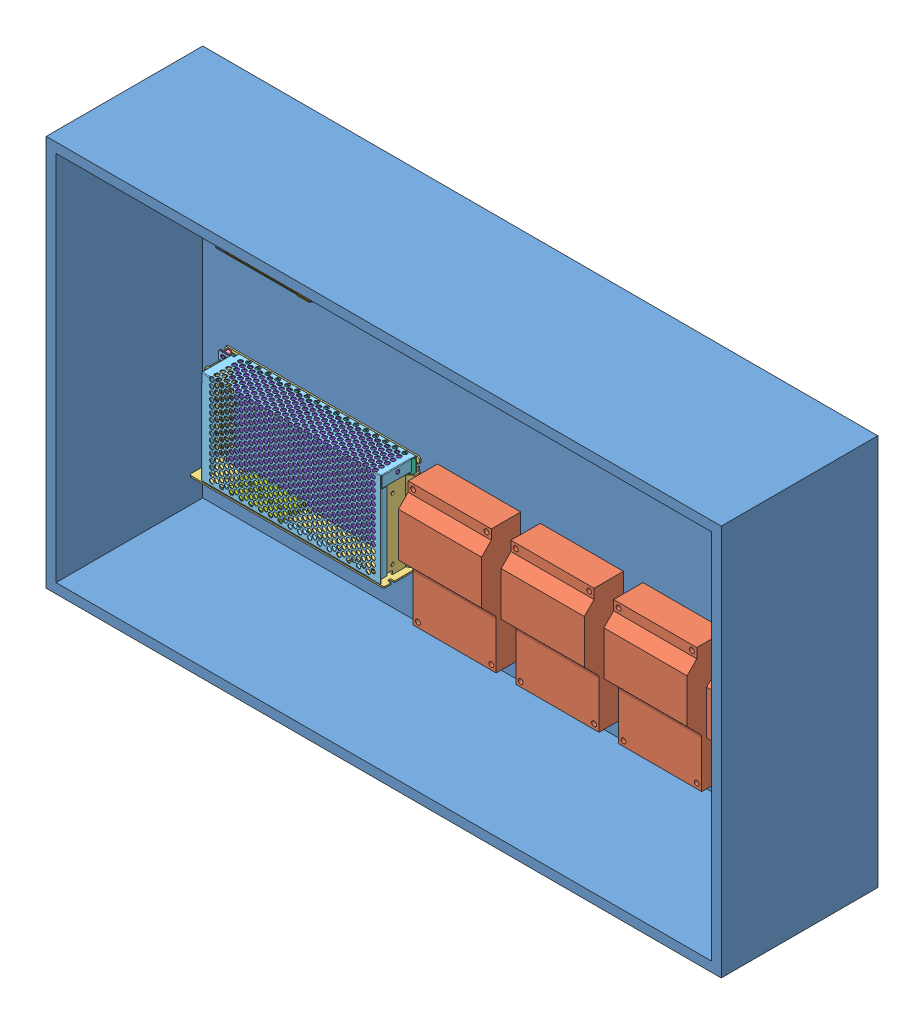
SolidWorks assembly quadro_elettrico_full, configuration Default. Lengths in mm.
Overall size (690 400 160).
33 component instances, 20 part files, 17 mates.
Components (placement in the parent):
- quadro_elettrico-1: quadro_elettrico [Default] at origin size (690 400 160)
- minitraction_power_mockup-1: minitraction_power_mockup [Default] at (-52.5 -105 10) size (85 130 40)
- SD-100C-12-1: SD-100C-12 [Default] at (-211.5 -91.125 11.5) x (1 0 0) z (0 -1 0) size (199.09 37.75 98.27)
  - SD-100C-12.stp-1: SD-100C-12.stp [Default] at origin size (199.09 37.75 98.27)
    - SD-100-20201028.stp.stp-1: SD-100-20201028.stp.stp [Default] at origin size (199.09 37.75 98.27)
      - SD-100_STP.ASM.stp-1: SD-100_STP.ASM.stp [Default] at origin size (199.09 37.75 98.27)
        - SD-100_1_ASM.ASM.stp-1: SD-100_1_ASM.ASM.stp [Default] at origin size (199 37.75 98.27)
          - 902-D-80_ASM.ASM.stp-1: 902-D-80_ASM.ASM.stp [Default] at origin size (199 37.75 97.75)
            - 902-D-119_PRT.PRT.stp-1: 902-D-119_PRT.PRT.stp [Default] at origin size (199 37.75 97.75)
            - NUT_PRT.PRT.stp-1: NUT_PRT.PRT.stp [Default] at (-111.528 -1.5 -40.7894) x (-1 0 0) z (0 1 0) size (8 6.93 6)
          - 902-T_PRT.PRT.stp-1: 902-T_PRT.PRT.stp [Default] at (96.5 36.1 -49.375) x (-1 0 0) z (0 0 -1) size (195.5 36.02 96.52)
          - MYLAR_PRT.PRT.stp-1: MYLAR_PRT.PRT.stp [Default] at (79.2081 1.5 46.5396) x (-1 0 0) z (0 -1 0) size (197 95 0.5)
          - HS2_PRT.PRT.stp-1: HS2_PRT.PRT.stp [Default] at (-64.5 -80.2586 -88.3567) x (0 0 1) z (-1 0 0) size (6.4 28 55)
          - PCB_PRT.PRT.stp-1: PCB_PRT.PRT.stp [Default] at (-189.5595 4.5 45.0362) x (1 0 0) z (0 1 0) size (194 95 1.6)
        - T44-BS1R05370120201023_STP.ASM.stp-1: T44-BS1R05370120201023_STP.ASM.stp [Default] at (-82.3888 6.1 -32.875) x (0 0 1) z (0 1 0) size (69.8 18 18.8)
          - 6_PRT.PRT.stp-1: 6_PRT.PRT.stp [Default] at origin size (7.51 7.5 3.96)
          - 2_PRT.PRT.stp-1: 2_PRT.PRT.stp [Default] at origin size (7.5 7.5 3.96)
          - 3_PRT.PRT.stp-1: 3_PRT.PRT.stp [Default] at origin size (7.51 7.5 3.96)
          - 4_PRT.PRT.stp-1: 4_PRT.PRT.stp [Default] at (0 0.8 0) size (69.8 18 18.8)
          - 5_PRT.PRT.stp-1: 5_PRT.PRT.stp [Default] at origin size (7.51 7.5 3.96)
          - 6_PRT_1.PRT.stp-1: 6_PRT_1.PRT.stp [Default] at (9.5 0 0) size (7.51 7.5 3.96)
          - 6_PRT_1_1.PRT.stp-1: 6_PRT_1_1.PRT.stp [Default] at (19 0 0) size (7.51 7.5 3.96)
          - 6_PRT_1_1_1.PRT.stp-1: 6_PRT_1_1_1.PRT.stp [Default] at (28.5 0 0) size (7.51 7.5 3.96)
- SD-25C-12-1: SD-25C-12 [Default] at (28.1917 -114.0246 17.8) size (99.05 97.03 36.06)
  - SD-25C-12.stp-1: SD-25C-12.stp [Default] at origin size (99.05 97.03 36.06)
    - RS-50_ASM_15.ASM.stp-1: RS-50_ASM_15.ASM.stp [Default] at origin size (99.05 97.03 36.06)
      - TN1_2.PRT.stp-1: TN1_2.PRT.stp [Default] at (-301.0065 335.8998 37.1723) x (0 0 -1) z (-1 0 0) size (15.25 49.25 14.66)
      - RS-50-CASE-T_21.PRT.stp-1: RS-50-CASE-T_21.PRT.stp [Default] at (0 1.5 1) size (97.05 96.6 36.06)
      - RS-50-CASE-D_28.PRT.stp-1: RS-50-CASE-D_28.PRT.stp [Default] at (-0.5 0.5 0) size (98.5 97 35)
      - RS-50-PCB_2.PRT.stp-1: RS-50-PCB_2.PRT.stp [Default] at (0 -0.6 -0.2033) size (98 95 1.6)
- minitraction_power_mockup-2: minitraction_power_mockup [Default] at (52.5 -105 10) size (85 130 40)
- minitraction_power_mockup-3: minitraction_power_mockup [Default] at (157.5 -105 10) size (85 130 40)
- minitraction_power_mockup-4: minitraction_power_mockup [Default] at (262.5 -105 10) size (85 130 40)
Mates (geometry in assembly coordinates):
- Coincidente1: coincident anti-aligned: plane of quadro_elettrico-1 through (0 0 10) normal (0 0 1); plane of minitraction_power_mockup-4 through (262.5 -105 10) normal (0 0 -1)
- Coincidente2: coincident anti-aligned: plane of quadro_elettrico-1 through (0 0 10) normal (0 0 1); plane of minitraction_power_mockup-3 through (157.5 -105 10) normal (0 0 -1)
- Coincidente3: coincident anti-aligned: plane of quadro_elettrico-1 through (0 0 10) normal (0 0 1); plane of minitraction_power_mockup-2 through (52.5 -105 10) normal (0 0 -1)
- Coincidente4: coincident anti-aligned: plane of quadro_elettrico-1 through (0 0 10) normal (0 0 1); plane of minitraction_power_mockup-1 through (-52.5 -105 10) normal (0 0 -1)
- Distanza1: distance = 20 mm anti-aligned: plane of minitraction_power_mockup-2 through (10 -40 50) normal (-1 0 0); plane of minitraction_power_mockup-1 through (-10 -40 50) normal (1 0 0)
- Coincidente6: coincident aligned: plane of minitraction_power_mockup-1 through (-95 -40 50) normal (0 1 0); plane of minitraction_power_mockup-2 through (10 -40 50) normal (0 1 0)
- Distanza2: distance = 20 mm anti-aligned: plane of minitraction_power_mockup-3 through (115 -40 50) normal (-1 0 0); plane of minitraction_power_mockup-2 through (95 -40 50) normal (1 0 0)
- Distanza3: distance = 20 mm anti-aligned: plane of minitraction_power_mockup-3 through (200 -40 50) normal (1 0 0); plane of minitraction_power_mockup-4 through (220 -40 50) normal (-1 0 0)
- Coincidente9: coincident aligned: plane of minitraction_power_mockup-3 through (115 -40 50) normal (0 1 0); plane of minitraction_power_mockup-4 through (220 -40 50) normal (0 1 0)
- Coincidente10: coincident aligned: plane of minitraction_power_mockup-2 through (10 -40 50) normal (0 1 0); plane of minitraction_power_mockup-3 through (115 -40 50) normal (0 1 0)
- Distanza4: distance = 30 mm anti-aligned: plane of minitraction_power_mockup-4 through (305 -40 50) normal (1 0 0); plane of quadro_elettrico-1 through (335 -190 160) normal (-1 0 0)
- Distanza5: distance = 20 mm anti-aligned: plane of minitraction_power_mockup-4 through (220 -170 50) normal (0 -1 0); plane of quadro_elettrico-1 through (-335 -190 160) normal (0 1 0)
- Coincidente11: coincident anti-aligned: plane of quadro_elettrico-1 through (0 0 10) normal (0 0 1); plane of SD-100C-12-1/SD-100C-12.stp-1/SD-100-20201028.stp.stp-1/SD-100_STP.ASM.stp-1/SD-100_1_ASM.ASM.stp-1/902-D-80_ASM.ASM.stp-1/902-D-119_PRT.PRT.stp-1 through (-211.5 -91.125 10) normal (0 0 -1)
- Distanza7: distance = 50 mm anti-aligned: plane of SD-100C-12-1/SD-100C-12.stp-1/SD-100-20201028.stp.stp-1/SD-100_STP.ASM.stp-1/SD-100_1_ASM.ASM.stp-1/902-D-80_ASM.ASM.stp-1/902-D-119_PRT.PRT.stp-1 through (-112 -140 10) normal (0 -1 0); plane of quadro_elettrico-1 through (-335 -190 160) normal (0 1 0)
- Distanza8: distance = 20 mm anti-aligned: plane of minitraction_power_mockup-1 through (-95 -40 50) normal (-1 0 0); plane of SD-100C-12-1/SD-100C-12.stp-1/SD-100-20201028.stp.stp-1/SD-100_STP.ASM.stp-1/SD-100_1_ASM.ASM.stp-1/902-T_PRT.PRT.stp-1 through (-115 -41.75 38.4938) normal (1 0 0)
- Distanza9: distance = 20 mm: plane of SD-25C-12-1/SD-25C-12.stp-1/RS-50_ASM_15.ASM.stp-1/RS-50-CASE-T_21.PRT.stp-1 through (-275.9748 170 12.5) normal (0 1 0); plane of quadro_elettrico-1 through (335 190 160) normal (0 -1 0)
- Coincidente12: coincident anti-aligned: plane of quadro_elettrico-1 through (0 0 10) normal (0 0 1); plane of SD-25C-12-1/SD-25C-12.stp-1/RS-50_ASM_15.ASM.stp-1/RS-50-CASE-D_28.PRT.stp-1 through (-140.7315 102.7505 114.0091) normal (0 0 -1)
